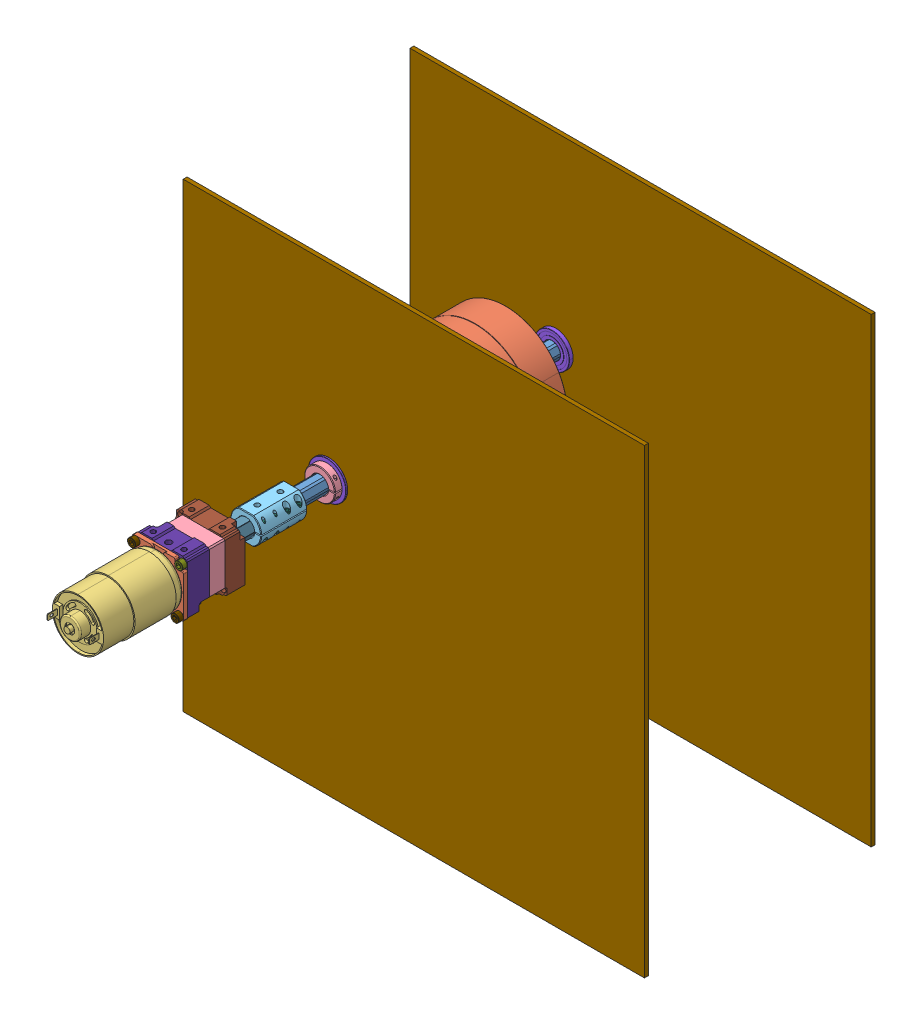
SolidWorks assembly Ramp and Flywheel, configuration Default. Lengths in mm.
Overall size (381 381 446).
65 component instances, 27 part files, 25 mates.
Components (placement in the parent):
- ThunderHex(.5 11inch)-SP-1: ThunderHex(.5 11inch)-SP [Default] at origin size (13.74 12.75 279.4)
- CompliantWheel(4inch 500)SP-1: CompliantWheel(4inch 500)SP [Default] at (15.9875 4.7838 39.3846) x (0.866025 0.5 0) z (0 0 1) size (101.6 101.6 25.4)
  - CompliantWheel(4inch 500)SP.STEP-1: CompliantWheel(4inch 500)SP.STEP [Default] at origin size (101.6 101.6 25.4)
    - 4IN Compliant Wheel FINAL Overmold.STEP-1: 4IN Compliant Wheel FINAL Overmold.STEP [Default] at (-16.2374 3.8509 18.652) size (101.6 101.6 25.4)
    - 2in Wheel Intergrated 0500 HEX Hub.STEP-1: 2in Wheel Intergrated 0500 HEX Hub.STEP [Default] at (-16.2374 3.8509 5.952) x (-1 0 0) z (0 0 -1) size (41.91 41.91 25.4)
- CompliantWheel(4inch 500)SP.STEP-1: CompliantWheel(4inch 500)SP.STEP [Default] at (15.9875 4.7838 64.7846) x (0.866025 0.5 0) z (0 0 1) size (101.6 101.6 25.4)
  - 4IN Compliant Wheel FINAL Overmold.STEP-1: 4IN Compliant Wheel FINAL Overmold.STEP [Default] at (-16.2374 3.8509 18.652) size (101.6 101.6 25.4)
  - 2in Wheel Intergrated 0500 HEX Hub.STEP-1: 2in Wheel Intergrated 0500 HEX Hub.STEP [Default] at (-16.2374 3.8509 5.952) x (-1 0 0) z (0 0 -1) size (41.91 41.91 25.4)
- CompliantWheel(4inch 500)SP.STEP-3: CompliantWheel(4inch 500)SP.STEP [Default] at (15.9875 4.7838 90.1846) x (0.866025 0.5 0) z (0 0 1) size (101.6 101.6 25.4)
  - 4IN Compliant Wheel FINAL Overmold.STEP-1: 4IN Compliant Wheel FINAL Overmold.STEP [Default] at (-16.2374 3.8509 18.652) size (101.6 101.6 25.4)
  - 2in Wheel Intergrated 0500 HEX Hub.STEP-1: 2in Wheel Intergrated 0500 HEX Hub.STEP [Default] at (-16.2374 3.8509 5.952) x (-1 0 0) z (0 0 -1) size (41.91 41.91 25.4)
- CompliantWheel(4inch 500)SP.STEP-4: CompliantWheel(4inch 500)SP.STEP [Default] at (15.9875 4.7838 115.5846) x (0.866025 0.5 0) z (0 0 1) size (101.6 101.6 25.4)
  - 4IN Compliant Wheel FINAL Overmold.STEP-1: 4IN Compliant Wheel FINAL Overmold.STEP [Default] at (-16.2374 3.8509 18.652) size (101.6 101.6 25.4)
  - 2in Wheel Intergrated 0500 HEX Hub.STEP-1: 2in Wheel Intergrated 0500 HEX Hub.STEP [Default] at (-16.2374 3.8509 5.952) x (-1 0 0) z (0 0 -1) size (41.91 41.91 25.4)
- ClampingShaftCollar(.5 in)SP-1: ClampingShaftCollar(.5 in)SP [Default] at (0 -0.2032 29.4616) size (25.39 25.4 6.35)
- ClampingShaftCollar(.5 in)SP-2: ClampingShaftCollar(.5 in)SP [Default] at (-0.8969 -0.0987 137.4116) size (25.39 25.4 6.35)
- Hex_Shaft_Coupler(.5)-SP-1: Hex_Shaft_Coupler(.5)-SP [Default] at (0.04 0 228.4754) size (25.76 22.32 38.1)
  - Hex_Shaft_Coupler(.5)-SP.STEP-1: Hex_Shaft_Coupler(.5)-SP.STEP [Default] at origin size (25.76 22.32 38.1)
    - 217-4008-001 Rev1.STEP-1: 217-4008-001 Rev1.STEP [Default] at origin size (25.38 10.66 38.1)
    - 217-4008-001 Rev1.STEP-2: 217-4008-001 Rev1.STEP [Default] x (1 0 0) z (0 0 -1) size (25.38 10.66 38.1)
    - 217-4008-002 Rev1_91251A108.STEP-1: 217-4008-002 Rev1_91251A108.STEP [Default] at (9.7928 7.025 4.7625) x (0.994016 0 -0.109231) z (0 1 0) size (4.65 4.65 12.38)
    - 217-4008-002 Rev1_91251A108.STEP-2: 217-4008-002 Rev1_91251A108.STEP [Default] at (9.7928 7.025 14.2875) x (-0.765668 0 -0.643235) z (0 1 0) size (4.65 4.65 12.38)
    - 217-4008-002 Rev1_91251A108.STEP-3: 217-4008-002 Rev1_91251A108.STEP [Default] at (-9.7928 7.025 14.2875) x (-0.114094 0 0.99347) z (0 1 0) size (4.65 4.65 12.38)
    - 217-4008-002 Rev1_91251A108.STEP-4: 217-4008-002 Rev1_91251A108.STEP [Default] at (-9.7928 7.025 4.7625) x (0.20346 0 0.979083) z (0 1 0) size (4.65 4.65 12.38)
    - 217-4008-002 Rev1_91251A108.STEP-5: 217-4008-002 Rev1_91251A108.STEP [Default] at (-9.7928 -7.025 -4.7625) x (0.20346 0 -0.979083) z (0 -1 0) size (4.65 4.65 12.38)
    - 217-4008-002 Rev1_91251A108.STEP-6: 217-4008-002 Rev1_91251A108.STEP [Default] at (-9.7928 -7.025 -14.2875) x (-0.114094 0 -0.99347) z (0 -1 0) size (4.65 4.65 12.38)
    - 217-4008-002 Rev1_91251A108.STEP-7: 217-4008-002 Rev1_91251A108.STEP [Default] at (9.7928 -7.025 -14.2875) x (-0.765668 0 0.643235) z (0 -1 0) size (4.65 4.65 12.38)
    - 217-4008-002 Rev1_91251A108.STEP-8: 217-4008-002 Rev1_91251A108.STEP [Default] at (9.7928 -7.025 -4.7625) x (0.994016 0 0.109231) z (0 -1 0) size (4.65 4.65 12.38)
- VersaPlanetaryv2_Single_Stage_10_1_with_775_Series (General_GearBox_Shell)-SP-1: VersaPlanetaryv2_Single_Stage_10_1_with_775_Series (General_GearBox_Shell)-SP [Default] at (0.0053 -22.165 285.8002) x (0 0 -1) z (1 0 0) size (166.6 49.04 49.3)
  - VersaPlanetary_v2_Single_Stage_10_1_with_775_Series (General_GearBox_Shell)-SP.STEP-1: VersaPlanetary_v2_Single_Stage_10_1_with_775_Series (General_GearBox_Shell)-SP.STEP [Default] at origin size (166.6 49.04 49.3)
    - 217-2820 Rev1_Public.STEP-1: 217-2820 Rev1_Public.STEP [Default] at (-4.6546 22.225 0) x (0 -0.456494 0.889726) z (-1 0 0) size (39.22 38.88 17.4)
      - 217-2625-100.STEP-1: 217-2625-100.STEP [Default] at origin size (39.22 38.88 12.7)
        - 217-2625-008 Rev1.STEP-1: 217-2625-008 Rev1.STEP [Default] at origin size (34.7 34.7 4.7)
        - 217-2625-010 Rev1.STEP-1: 217-2625-010 Rev1.STEP [Default] at (0 10.193 3.65) x (0.999813 0.019336 0) z (0 0 1) size (4 4 12)
        - 217-2625-010 Rev1.STEP-2: 217-2625-010 Rev1.STEP [Default] at (8.691 -5.3258 3.65) size (4 4 12)
        - 217-2625-010 Rev1.STEP-3: 217-2625-010 Rev1.STEP [Default] at (-8.691 -5.3258 3.65) size (4 4 12)
        - 217-2625-005 Rev1_Planet_Revolving_Follower01.STEP-1: 217-2625-005 Rev1_Planet_Revolving_Follower01.STEP [Default] at (8.691 -5.3258 6.35) x (0.932816 0.360354 0) z (0 0 1) size (16.89 16.89 8)
        - 217-2625-005 Rev1_Planet_Revolving_Follower01.STEP-2: 217-2625-005 Rev1_Planet_Revolving_Follower01.STEP [Default] at (-8.691 -5.3258 6.35) x (-0.932788 -0.360426 0) z (0 0 1) size (16.89 16.89 8)
        - 217-2625-005 Rev1_Planet_Revolving_Follower01.STEP-3: 217-2625-005 Rev1_Planet_Revolving_Follower01.STEP [Default] at (0 10.193 6.35) x (0.893583 0.448898 0) z (0 0 1) size (16.89 16.89 8)
      - 217-2625-007 Rev1_Public.STEP-1: 217-2625-007 Rev1_Public.STEP [Default] at (0 0 6.7) x (0.992772 0.120019 0) z (0 0 1) size (15.27 15.27 12.7)
    - 217-2625-026 Rev1.STEP-1: 217-2625-026 Rev1.STEP [Default] at (-6.5 22.225 0) x (0 -1 0) z (-1 0 0) size (44.45 42 18.12)
    - 217-2742-001 Rev4.STEP-1: 217-2742-001 Rev4.STEP [Default] at (0.2002 22.225 0) x (1 0 0) z (0 -0.092627 0.995701) size (7 28 28)
    - 217-2742-001 Rev4.STEP-2: 217-2742-001 Rev4.STEP [Default] at (8.2002 22.225 0) size (7 28 28)
    - 217-2625-017 Rev1_9714K61.STEP-1: 217-2625-017 Rev1_9714K61.STEP [Default] at (7.42 22.3002 -0.342) x (0 0.56703 0.823697) z (0 -0.823697 0.56703) size (28.51 4.98 27.43)
    - 217-2625-003 Rev1.STEP-1: 217-2625-003 Rev1.STEP [Default] at (7.4478 22.225 0) x (0 -1 0) z (1 0 0) size (17 17 64.11)
    - 217-2625-018 Rev1_98541A410.STEP-1: 217-2625-018 Rev1_98541A410.STEP [Default] at (-0.7046 22.225 0) x (1 0 0) z (0 -0.017452 0.999848) size (1 19.6 17.4)
    - 832-1750-Ring-Gear-Screw_SSA0832-0500ZC.STEP-1: 832-1750-Ring-Gear-Screw_SSA0832-0500ZC.STEP [Default] at (-30.7 4.725 -17.5) x (0 0.997447 0.071411) z (0 -0.071411 0.997447) size (6.73 48.51 6.73)
    - 832-1750-Ring-Gear-Screw_SSA0832-0500ZC.STEP-2: 832-1750-Ring-Gear-Screw_SSA0832-0500ZC.STEP [Default] at (-30.7 39.725 17.5) x (0 0.005929 0.999982) z (0 -0.999982 0.005929) size (6.73 48.51 6.73)
    - 217-2625-025 Rev1.STEP-1: 217-2625-025 Rev1.STEP [Default] at (-23.2 22.225 0) x (0 -1 0) z (-1 0 0) size (44.45 42 18)
    - 217-4649-002 Rev1_SSA0832-0500ZC.STEP-1: 217-4649-002 Rev1_SSA0832-0500ZC.STEP [Default] at (-34.2 4.2645 17.9605) x (0 0.33842 -0.940995) z (0 0.940995 0.33842) size (6.73 16.76 6.73)
    - 217-4649-002 Rev1_SSA0832-0500ZC.STEP-2: 217-4649-002 Rev1_SSA0832-0500ZC.STEP [Default] at (-34.2 40.1855 -17.9605) x (0 -0.308932 -0.951084) z (0 0.951084 -0.308932) size (6.73 16.76 6.73)
    - 217-4649-006 Rev1_SSA0004-008BA.STEP-1: 217-4649-006 Rev1_SSA0004-008BA.STEP [Default] at (-30.7 22.225 14.5) x (0 0.5 -0.866025) z (0 -0.866025 -0.5) size (7 14 7)
    - 217-4649-006 Rev1_SSA0004-008BA.STEP-2: 217-4649-006 Rev1_SSA0004-008BA.STEP [Default] at (-30.7 22.225 -14.5) x (0 -1 0) z (0 0 1) size (7 14 7)
    - 217-2822-002 Rev4.STEP-1: 217-2822-002 Rev4.STEP [Default] at (-32.45 22.225 0) x (0 -1 0) z (-1 0 0) size (42 42 5.3)
    - 217-4347-000 Rev1.STEP-1: 217-4347-000 Rev1.STEP [Default] at (-34.2 22.225 0) x (-1 0 0) z (0 1 0) size (88 44.3 44.3)
    - 217-2816-001 Rev1.STEP-1: 217-2816-001 Rev1.STEP [Default] at (-6.35 22.225 0) x (0 -1 0) z (1 0 0) size (42 42 14.51)
    - 217-4649-001 Rev1.STEP-1: 217-4649-001 Rev1.STEP [Default] at (-20.554 22.225 0) x (0 -1 0) z (1 0 0) size (18 18 13)
    - 217-4649-007 Rev1_94105A824.STEP-1: 217-4649-007 Rev1_94105A824.STEP [Default] at (-26.029 22.225 -6.7835) x (-0.996104 -0.088191 0) z (0 0 -1) size (4.83 4.83 4.77)
    - 217-2625-013 Rev2.STEP-1: 217-2625-013 Rev2.STEP [Default] at (-25.2898 22.225 0) x (0 0 1) z (-1 0 0) size (8.01 7.94 7.5)
- 13_75mm_1_2_ThunderHex_ID_x_1_125_OD_x_0_313_WD_Flanged_Bearing_217-4006.step-1: 13_75mm_1_2_ThunderHex_ID_x_1_125_OD_x_0_313_WD_Flanged_Bearing_217-4006.step [Default] at (0 0 -9.4322) x (-1 0 0) z (0 0 -1) size (31.12 31.12 7.94)
- 13_75mm_1_2_ThunderHex_ID_x_1_125_OD_x_0_313_WD_Flanged_Bearing_217-4006.step-2: 13_75mm_1_2_ThunderHex_ID_x_1_125_OD_x_0_313_WD_Flanged_Bearing_217-4006.step [Default] at (0.0358 -0.0294 176.3566) x (-1 -0.000016 0) z (0 0 1) size (31.12 31.12 7.94)
- ClampingShaftCollar(.5 in)SP-3: ClampingShaftCollar(.5 in)SP [Default] at (0.1173 0 -16.3259) size (25.39 25.4 6.35)
- ClampingShaftCollar(.5 in)SP-4: ClampingShaftCollar(.5 in)SP [Default] at (-0.0587 -0.1016 183.2503) size (25.39 25.4 6.35)
- Wall(15 by 15 in .125thickness)-SP-1: Wall(15 by 15 in .125thickness)-SP [Default] at (13.4793 -64.9577 -8.6384) x (0 0 -1) z (1 0 0) size (3.17 381 381)
- Wall(15 by 15 in .125thickness)-SP-2: Wall(15 by 15 in .125thickness)-SP [Default] at (13.4793 -64.9577 178.7378) x (0 0 -1) z (1 0 0) size (3.17 381 381)
Mates (geometry in assembly coordinates):
- Coincident1: coincident: plane of ThunderHex(.5 11inch)-SP-1 through (-3.6808 6.3754 228.6) normal (-0.866025 0.5 0); plane of CompliantWheel(4inch 500)SP-1/CompliantWheel(4inch 500)SP.STEP-1/2in Wheel Intergrated 0500 HEX Hub.STEP-1 through (-3.6808 6.3754 32.6366) normal (0.866025 -0.5 0)
- Coincident2: coincident: plane of ThunderHex(.5 11inch)-SP-1 through (3.6808 6.3754 228.6) normal (0 1 0); plane of CompliantWheel(4inch 500)SP-1/CompliantWheel(4inch 500)SP.STEP-1/2in Wheel Intergrated 0500 HEX Hub.STEP-1 through (3.6808 6.3754 32.6366) normal (0 -1 0)
- Coincident3: coincident: circle of CompliantWheel(4inch 500)SP-1/CompliantWheel(4inch 500)SP.STEP-1/2in Wheel Intergrated 0500 HEX Hub.STEP-1; plane of CompliantWheel(4inch 500)SP.STEP-1/2in Wheel Intergrated 0500 HEX Hub.STEP-1 through (-1.27 2.1997 58.0366) normal (0 0 -1)
- Coincident4: coincident: circle of CompliantWheel(4inch 500)SP.STEP-1/4IN Compliant Wheel FINAL Overmold.STEP-1; plane of CompliantWheel(4inch 500)SP.STEP-3/2in Wheel Intergrated 0500 HEX Hub.STEP-1 through (-1.27 2.1997 83.4366) normal (0 0 -1)
- Coincident5: coincident: circle of CompliantWheel(4inch 500)SP.STEP-3/2in Wheel Intergrated 0500 HEX Hub.STEP-1; plane of CompliantWheel(4inch 500)SP.STEP-4/2in Wheel Intergrated 0500 HEX Hub.STEP-1 through (-1.27 2.1997 108.8366) normal (0 0 -1)
- Coincident7: coincident: plane of CompliantWheel(4inch 500)SP-1/CompliantWheel(4inch 500)SP.STEP-1/2in Wheel Intergrated 0500 HEX Hub.STEP-1 through (-1.27 2.1997 32.6366) normal (0 0 -1); plane of ClampingShaftCollar(.5 in)SP-1 through (0 -0.2032 32.6366) normal (0 0 1)
- Coincident8: coincident: plane of ThunderHex(.5 11inch)-SP-1 through (-3.6808 6.3754 228.6) normal (-0.866025 0.5 0); plane of ClampingShaftCollar(.5 in)SP-1 through (-3.7395 6.2738 26.2866) normal (0.866025 -0.5 0)
- Coincident9: coincident: plane of ThunderHex(.5 11inch)-SP-1 through (7.3617 0 228.6) normal (0.866025 0.5 0); plane of ClampingShaftCollar(.5 in)SP-1 through (7.479 -0.2032 26.2866) normal (-0.866025 -0.5 0)
- Coincident13: coincident: plane of CompliantWheel(4inch 500)SP.STEP-4/2in Wheel Intergrated 0500 HEX Hub.STEP-1 through (-1.27 2.1997 134.2366) normal (0 0 1); plane of ClampingShaftCollar(.5 in)SP-2 through (-0.8969 -0.0987 134.2366) normal (0 0 -1)
- Coincident16: coincident: plane of ThunderHex(.5 11inch)-SP-1 through (0 0 228.6) normal (0 0 1); plane of VersaPlanetaryv2_Single_Stage_10_1_with_775_Series (General_GearBox_Shell)-SP-1/VersaPlanetary_v2_Single_Stage_10_1_with_775_Series (General_GearBox_Shell)-SP.STEP-1/217-2625-003 Rev1.STEP-1 through (3.6715 6.41 228.6) normal (0 0 -1)
- Coincident17: coincident: plane of ThunderHex(.5 11inch)-SP-1 through (-7.3617 0 228.6) normal (-0.866025 -0.5 0); plane of Hex_Shaft_Coupler(.5)-SP-1/Hex_Shaft_Coupler(.5)-SP.STEP-1/217-4008-001 Rev1.STEP-2 through (-3.6609 -6.41 247.5254) normal (0.866025 0.5 0)
- Coincident18: coincident: plane of ThunderHex(.5 11inch)-SP-1 through (-3.6808 6.3754 228.6) normal (-0.866025 0.5 0); plane of Hex_Shaft_Coupler(.5)-SP-1/Hex_Shaft_Coupler(.5)-SP.STEP-1/217-4008-001 Rev1.STEP-1 through (-3.6609 6.41 209.4254) normal (0.866025 -0.5 0)
- Coincident21: coincident: plane of Hex_Shaft_Coupler(.5)-SP-1/Hex_Shaft_Coupler(.5)-SP.STEP-1/217-4008-001 Rev1.STEP-1 through (-3.6609 6.41 209.4254) normal (0.866025 -0.5 0); plane of VersaPlanetaryv2_Single_Stage_10_1_with_775_Series (General_GearBox_Shell)-SP-1/VersaPlanetary_v2_Single_Stage_10_1_with_775_Series (General_GearBox_Shell)-SP.STEP-1/217-2625-003 Rev1.STEP-1 through (-7.327 0.06 228.6) normal (-0.866025 0.5 0)
- Coincident22: coincident: plane of Hex_Shaft_Coupler(.5)-SP-1/Hex_Shaft_Coupler(.5)-SP.STEP-1/217-4008-001 Rev1.STEP-1 through (3.7408 6.41 209.4254) normal (0 -1 0); plane of VersaPlanetaryv2_Single_Stage_10_1_with_775_Series (General_GearBox_Shell)-SP-1/VersaPlanetary_v2_Single_Stage_10_1_with_775_Series (General_GearBox_Shell)-SP.STEP-1/217-2625-003 Rev1.STEP-1 through (-3.6609 6.41 228.6) normal (0 1 0)
- Concentric2: concentric: circle of ThunderHex(.5 11inch)-SP-1; circle of 13_75mm_1_2_ThunderHex_ID_x_1_125_OD_x_0_313_WD_Flanged_Bearing_217-4006.step-1
- Distance1: distance = 31.75 mm: plane of ClampingShaftCollar(.5 in)SP-1 through (0 -0.2032 26.2866) normal (0 0 -1); plane of 13_75mm_1_2_ThunderHex_ID_x_1_125_OD_x_0_313_WD_Flanged_Bearing_217-4006.step-1 through (0 6.875 -5.4634) normal (0 0 1)
- Coincident25: coincident: plane of 13_75mm_1_2_ThunderHex_ID_x_1_125_OD_x_0_313_WD_Flanged_Bearing_217-4006.step-1 through (0 12.2875 -13.1509) normal (0 0 -1); plane of ClampingShaftCollar(.5 in)SP-3 through (0.1173 0 -13.1509) normal (0 0 1)
- Coincident26: coincident: plane of ThunderHex(.5 11inch)-SP-1 through (-3.6808 6.3754 228.6) normal (-0.866025 0.5 0); plane of ClampingShaftCollar(.5 in)SP-3 through (-3.6222 6.477 -19.5009) normal (0.866025 -0.5 0)
- Coincident27: coincident: plane of ThunderHex(.5 11inch)-SP-1 through (-7.3617 0 228.6) normal (-0.866025 -0.5 0); plane of ClampingShaftCollar(.5 in)SP-3 through (-7.3617 0 -19.5009) normal (0.866025 0.5 0)
- Coincident28: coincident: plane of 13_75mm_1_2_ThunderHex_ID_x_1_125_OD_x_0_313_WD_Flanged_Bearing_217-4006.step-2 through (0.036 -12.3169 180.0753) normal (0 0 1); plane of ClampingShaftCollar(.5 in)SP-4 through (-0.0587 -0.1016 180.0753) normal (0 0 -1)
- Coincident30: coincident: plane of ThunderHex(.5 11inch)-SP-1 through (7.3617 0 228.6) normal (0.866025 0.5 0); plane of ClampingShaftCollar(.5 in)SP-4 through (7.4203 -0.1016 180.0753) normal (-0.866025 -0.5 0)
- Coincident31: coincident: plane of ThunderHex(.5 11inch)-SP-1 through (3.6808 6.3754 228.6) normal (0 1 0); plane of ClampingShaftCollar(.5 in)SP-4 through (3.6808 6.3754 180.0753) normal (0 -1 0)
- Coincident32: coincident: plane of 13_75mm_1_2_ThunderHex_ID_x_1_125_OD_x_0_313_WD_Flanged_Bearing_217-4006.step-1 through (0 14.2875 -11.8134) normal (0 0 1); plane of Wall(15 by 15 in .125thickness)-SP-1 through (13.4793 -64.9577 -11.8134) normal (0 0 -1)
- Lock1: lock: unknown of 13_75mm_1_2_ThunderHex_ID_x_1_125_OD_x_0_313_WD_Flanged_Bearing_217-4006.step-2; unknown of Wall(15 by 15 in .125thickness)-SP-2
- Coincident34: coincident: plane of 13_75mm_1_2_ThunderHex_ID_x_1_125_OD_x_0_313_WD_Flanged_Bearing_217-4006.step-2 through (0.036 -14.3169 178.7378) normal (0 0 -1); plane of Wall(15 by 15 in .125thickness)-SP-2 through (13.4793 -64.9577 178.7378) normal (0 0 1)
